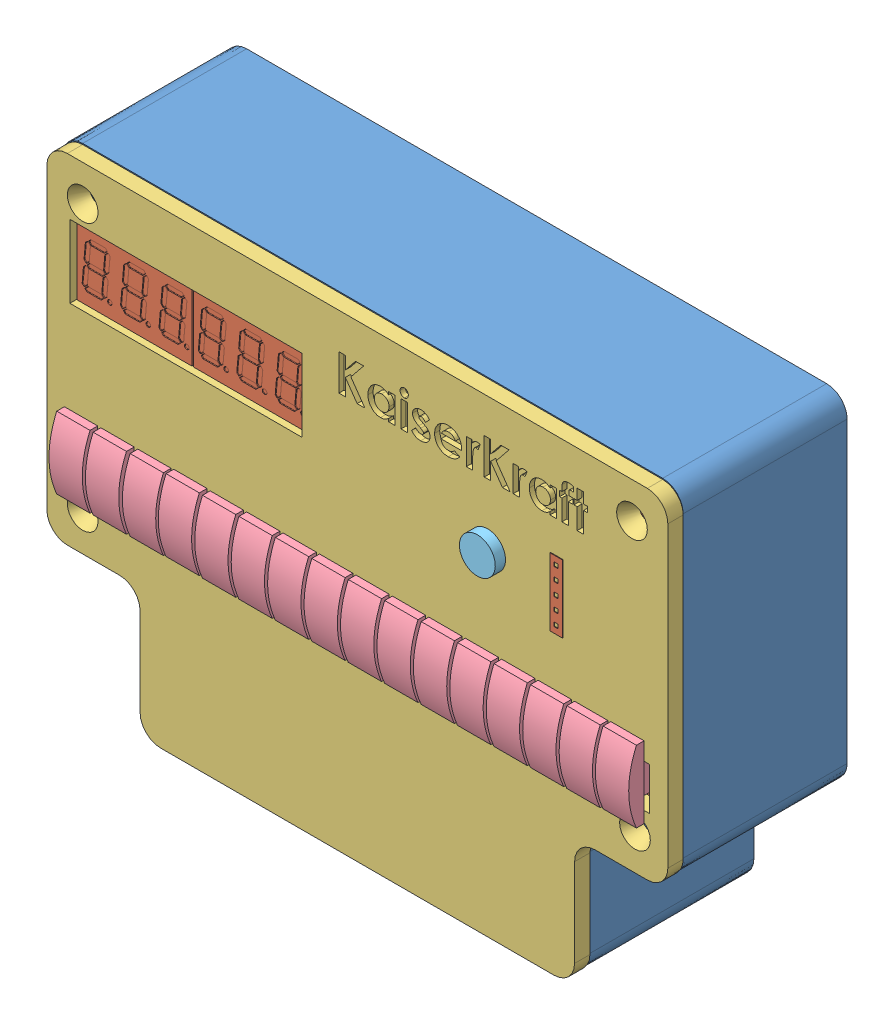
SolidWorks assembly submission, configuration Domyślna. Lengths in mm.
Overall size (121.28 91.6 38.61).
21 component instances, 6 part files, 60 mates.
Components (placement in the parent):
- Bottom_part-1: Bottom_part [Domyślna] x (-1 0 0) z (0 0 -1) size (121.2 91.4 32)
- Calculator.step-2: Calculator.step [Domyślna] at (-115.2 -0.196 -5.3886) size (120.85 86.07 32.47)
- Top_part-1: Top_part [Domyślna] at origin size (121.2 91.4 3)
- Switch_part-1: Switch_part [Domyślna] at (-111.9619 14.572 -0.3886) x (1 0 0) z (0 0 1) size (6.5 14 7)
- Switch_part-2: Switch_part [Domyślna] at (-104.8499 14.572 -0.3886) x (1 0 0) z (0 0 1) size (6.5 14 7)
- Button_top-1: Button_top [Domyślna] at (-31.5 37.75 5.6799) x (0.247537 0.968879 0) z (0 0 -1) size (7 7 6)
- Button_bottom-1: Button_bottom [Domyślna] at (-31.5 37.75 -0.3201) x (0.962619 -0.270858 0) z (0 0 1) size (5 5 2)
- Switch_part-5: Switch_part [Domyślna] at (-97.6379 14.572 -0.3886) x (1 0 0) z (0 0 1) size (6.5 14 7)
- Switch_part-6: Switch_part [Domyślna] at (-90.6259 14.672 -0.3886) x (1 0 0) z (0 0 1) size (6.5 14 7)
- Switch_part-7: Switch_part [Domyślna] at (-83.5139 14.572 -0.3886) x (1 0 0) z (0 0 1) size (6.5 14 7)
- Switch_part-8: Switch_part [Domyślna] at (-76.4019 14.572 -0.3886) x (1 0 0) z (0 0 1) size (6.5 14 7)
- Switch_part-9: Switch_part [Domyślna] at (-69.2899 14.572 -0.3886) x (1 0 0) z (0 0 1) size (6.5 14 7)
- Switch_part-10: Switch_part [Domyślna] at (-62.1779 14.572 -0.3886) x (1 0 0) z (0 0 1) size (6.5 14 7)
- Switch_part-11: Switch_part [Domyślna] at (-55.0659 14.572 -0.3886) x (1 0 0) z (0 0 1) size (6.5 14 7)
- Switch_part-12: Switch_part [Domyślna] at (-47.9539 14.572 -0.3886) x (1 0 0) z (0 0 1) size (6.5 14 7)
- Switch_part-13: Switch_part [Domyślna] at (-40.8419 14.572 -0.3886) x (1 0 0) z (0 0 1) size (6.5 14 7)
- Switch_part-14: Switch_part [Domyślna] at (-33.7299 14.572 -0.3886) x (1 0 0) z (0 0 1) size (6.5 14 7)
- Switch_part-15: Switch_part [Domyślna] at (-26.6179 14.572 -0.3886) x (1 0 0) z (0 0 1) size (6.5 14 7)
- Switch_part-16: Switch_part [Domyślna] at (-19.5059 14.572 -0.3886) x (1 0 0) z (0 0 1) size (6.5 14 7)
- Switch_part-17: Switch_part [Domyślna] at (-12.3939 14.572 -0.3886) x (1 0 0) z (0 0 1) size (6.5 14 7)
- Switch_part-18: Switch_part [Domyślna] at (-5.3219 14.672 -0.3886) x (1 0 0) z (0 0 1) size (6.5 14 7)
Mates (geometry in assembly coordinates):
- Wspólnie1: coincident: plane of Calculator.step-1 through (-48.0898 -16.8983 120.85) normal (0 0 1); circle of Bottom_part-1
- Wspólnie2: coincident: plane of Calculator.step-1 through (-48.0898 43.0977 120.4385) normal (-1 0 0); plane of Bottom_part-1 through (-115.2 60.2 -29) normal (1 0 0)
- Wspólnie3: coincident anti-aligned: plane of Calculator.step-1 through (66.9062 43.0977 120.4385) normal (0 1 0); plane of Bottom_part-1 through (0 60.2 -29) normal (0 -1 0)
- Ustalone2: in place: plane of ? through (66.9102 -16.9023 122.45) normal (0 0 1); plane of ? through (0 0 122.45) normal (0 0 1); moOrthogonalPlaneRef_w of ? through (66.9102 -16.9023 122.45) normal (0 0 1); plane of ? through (0 0 122.45) normal (0 1 0); plane of ? through (66.9102 -16.9023 122.45) normal (0 0 1); plane of ? through (0 0 122.45) normal (1 0 0); plane of Bottom_part-1 through (0 0 0) normal (0 0 1); unknown of Top_part-1
- Wspólnie9: coincident aligned: plane of Bottom_part-1; plane of Top_part-1
- Wspólnie10: coincident aligned: moOrthogonalPlaneRef_w of Bottom_part-1 through (0 0 0) normal (0 1 0); plane of Część6^submission-1 through (0 0 0) normal (0 1 0)
- Wspólnie11: coincident anti-aligned: moOrthogonalPlaneRef_w of Bottom_part-1 through (0 0 0) normal (-1 0 0); plane of Część6^submission-1 through (0 0 0) normal (1 0 0)
- Wspólnie18: coincident anti-aligned: plane of Bottom_part-1 through (-3.9013 56.1037 -7) normal (0 0 1); plane of Calculator.step-2 through (-115.2 -0.196 -7) normal (0 0 -1)
- Wspólnie19: coincident anti-aligned: plane of Bottom_part-1 through (-97 -25.2 -29) normal (0 1 0); plane of Calculator.step-2 through (-97.2 -25.2 -7) normal (0 -1 0)
- Wspólnie20: coincident: plane of Bottom_part-1 through (-115.2 60.2 -29) normal (1 0 0); line of Calculator.step-2 through (-115.2 59.8 -5.3886) axis (0 -1 0)
- Wspólnie21: coincident anti-aligned: plane of Calculator.step-2 through (-109.8619 17.1354 -0.3886) normal (1 0 0); plane of Switch_part-1 through (-109.8619 14.572 3.6114) normal (-1 0 0)
- Wspólnie24: coincident anti-aligned: plane of Calculator.step-2 through (-111.8619 13.072 3.6114) normal (0 0 1); plane of Switch_part-1 through (-111.9619 14.572 3.6114) normal (0 0 -1)
- Wspólnie25: coincident anti-aligned: plane of Calculator.step-2 through (-111.8619 14.572 -1.3886) normal (0 1 0); plane of Switch_part-1 through (-111.9619 14.572 3.6114) normal (0 -1 0)
- Wspólnie26: coincident anti-aligned: plane of Calculator.step-2 through (-102.7499 17.1354 -0.3886) normal (1 0 0); plane of Switch_part-2 through (-102.7499 14.572 3.6114) normal (-1 0 0)
- Wspólnie27: coincident anti-aligned: plane of Calculator.step-2 through (-104.7499 13.072 3.6114) normal (0 0 1); plane of Switch_part-2 through (-104.8499 14.572 3.6114) normal (0 0 -1)
- Wspólnie28: coincident anti-aligned: plane of Calculator.step-2 through (-104.7499 14.572 -1.3886) normal (0 1 0); plane of Switch_part-2 through (-104.8499 14.572 3.6114) normal (0 -1 0)
- Koncentryczne3: concentric anti-aligned: cylinder of Top_part-1 through (-31.5 37.75 0) axis (0 0 1) radius 1.6; cylinder of Button_bottom-1 through (-31.5 37.75 1.6799) axis (0 0 -1) radius 1.5
- Koncentryczne4: concentric anti-aligned: cylinder of Top_part-1 through (-31.5 37.75 0) axis (0 0 1) radius 1.6; circle of Button_top-1
- Wspólnie29: coincident aligned: circle of Button_top-1; plane of Button_bottom-1 through (-31.5 37.75 -0.3201) normal (0 0 -1)
- Wspólnie30: coincident anti-aligned: plane of Calculator.step-2 through (-97.6379 14.572 -1.3886) normal (0 1 0); plane of Switch_part-3 through (-82.5484 14.572 10.5) normal (0 -1 0)
- Wspólnie33: coincident anti-aligned: plane of Calculator.step-2 through (-96.2263 17.1354 -0.3886) normal (0 0 1); plane of Switch_part-5 through (-97.6379 14.572 -0.3886) normal (0 0 -1)
- Wspólnie34: coincident anti-aligned: plane of Calculator.step-2 through (-89.1143 17.1354 -0.3886) normal (0 0 1); plane of Switch_part-6 through (-90.6259 14.672 -0.3886) normal (0 0 -1)
- Wspólnie35: coincident anti-aligned: plane of Calculator.step-2 through (-82.0023 17.1354 -0.3886) normal (0 0 1); plane of Switch_part-7 through (-83.5139 14.572 -0.3886) normal (0 0 -1)
- Wspólnie38: coincident anti-aligned: plane of Calculator.step-2 through (-90.5259 12.572 3.6114) normal (0 -1 0); plane of Switch_part-6 through (-90.6259 12.572 3.6114) normal (0 1 0)
- Wspólnie39: coincident anti-aligned: plane of Calculator.step-2 through (-88.5259 17.1354 -0.3886) normal (1 0 0); plane of Switch_part-6 through (-88.5259 14.672 3.6114) normal (-1 0 0)
- Wspólnie41: coincident anti-aligned: plane of Calculator.step-2 through (-81.4139 17.1354 -0.3886) normal (1 0 0); plane of Switch_part-7 through (-81.4139 14.572 3.6114) normal (-1 0 0)
- Wspólnie42: coincident anti-aligned: plane of Calculator.step-2 through (-83.4139 14.572 -1.3886) normal (0 1 0); plane of Switch_part-7 through (-83.5139 14.572 3.6114) normal (0 -1 0)
- Wspólnie77: coincident anti-aligned: plane of Calculator.step-2 through (-3.8103 17.1354 -0.3886) normal (0 0 1); plane of Switch_part-18 through (-5.3219 14.672 -0.3886) normal (0 0 -1)
- Wspólnie78: coincident anti-aligned: plane of Calculator.step-2 through (-3.8103 17.1354 -0.3886) normal (0 0 1); plane of Switch_part-17 through (-12.3939 14.572 -0.3886) normal (0 0 -1)
- Wspólnie80: coincident anti-aligned: plane of Calculator.step-2 through (-3.8103 17.1354 -0.3886) normal (0 0 1); plane of Switch_part-16 through (-19.5059 14.572 -0.3886) normal (0 0 -1)
- Wspólnie81: coincident anti-aligned: plane of Calculator.step-2 through (-3.8103 17.1354 -0.3886) normal (0 0 1); plane of Switch_part-15 through (-26.6179 14.572 -0.3886) normal (0 0 -1)
- Wspólnie82: coincident anti-aligned: plane of Calculator.step-2 through (-3.8103 17.1354 -0.3886) normal (0 0 1); plane of Switch_part-14 through (-33.7299 14.572 -0.3886) normal (0 0 -1)
- Wspólnie83: coincident anti-aligned: plane of Calculator.step-2 through (-3.8103 17.1354 -0.3886) normal (0 0 1); plane of Switch_part-13 through (-40.8419 14.572 -0.3886) normal (0 0 -1)
- Wspólnie84: coincident anti-aligned: plane of Calculator.step-2 through (-3.8103 17.1354 -0.3886) normal (0 0 1); plane of Switch_part-12 through (-47.9539 14.572 -0.3886) normal (0 0 -1)
- Wspólnie85: coincident anti-aligned: plane of Calculator.step-2 through (-3.8103 17.1354 -0.3886) normal (0 0 1); plane of Switch_part-11 through (-55.0659 14.572 -0.3886) normal (0 0 -1)
- Wspólnie86: coincident anti-aligned: plane of Calculator.step-2 through (-3.8103 17.1354 -0.3886) normal (0 0 1); plane of Switch_part-10 through (-62.1779 14.572 -0.3886) normal (0 0 -1)
- Wspólnie87: coincident anti-aligned: plane of Calculator.step-2 through (-3.8103 17.1354 -0.3886) normal (0 0 1); plane of Switch_part-8 through (-76.4019 14.572 -0.3886) normal (0 0 -1)
- Wspólnie88: coincident anti-aligned: plane of Calculator.step-2 through (-3.8103 17.1354 -0.3886) normal (0 0 1); plane of Switch_part-9 through (-69.2899 14.572 -0.3886) normal (0 0 -1)
- Wspólnie89: coincident anti-aligned: plane of Calculator.step-2 through (-3.2219 17.1354 -0.3886) normal (1 0 0); plane of Switch_part-18 through (-3.2219 14.672 3.6114) normal (-1 0 0)
- Wspólnie90: coincident anti-aligned: plane of Calculator.step-2 through (-10.2939 17.1354 -0.3886) normal (1 0 0); plane of Switch_part-17 through (-10.2939 14.572 3.6114) normal (-1 0 0)
- Wspólnie91: coincident anti-aligned: plane of Calculator.step-2 through (-17.4059 17.1354 -0.3886) normal (1 0 0); plane of Switch_part-16 through (-17.4059 14.572 3.6114) normal (-1 0 0)
- Wspólnie92: coincident anti-aligned: plane of Calculator.step-2 through (-24.5179 17.1354 -0.3886) normal (1 0 0); plane of Switch_part-15 through (-24.5179 14.572 3.6114) normal (-1 0 0)
- Wspólnie93: coincident anti-aligned: plane of Calculator.step-2 through (-31.6299 17.1354 -0.3886) normal (1 0 0); plane of Switch_part-14 through (-31.6299 14.572 3.6114) normal (-1 0 0)
- Wspólnie94: coincident anti-aligned: plane of Calculator.step-2 through (-38.7419 17.1354 -0.3886) normal (1 0 0); plane of Switch_part-13 through (-38.7419 14.572 3.6114) normal (-1 0 0)
- Wspólnie95: coincident anti-aligned: plane of Calculator.step-2 through (-45.8539 17.1354 -0.3886) normal (1 0 0); plane of Switch_part-12 through (-45.8539 14.572 3.6114) normal (-1 0 0)
- Wspólnie96: coincident anti-aligned: plane of Calculator.step-2 through (-52.9659 17.1354 -0.3886) normal (1 0 0); plane of Switch_part-11 through (-52.9659 14.572 3.6114) normal (-1 0 0)
- Wspólnie97: coincident anti-aligned: plane of Calculator.step-2 through (-60.0779 17.1354 -0.3886) normal (1 0 0); plane of Switch_part-10 through (-60.0779 14.572 3.6114) normal (-1 0 0)
- Wspólnie98: coincident anti-aligned: plane of Calculator.step-2 through (-67.1899 17.1354 -0.3886) normal (1 0 0); plane of Switch_part-9 through (-67.1899 14.572 3.6114) normal (-1 0 0)
- Wspólnie99: coincident anti-aligned: plane of Calculator.step-2 through (-74.3019 17.1354 -0.3886) normal (1 0 0); plane of Switch_part-8 through (-74.3019 14.572 3.6114) normal (-1 0 0)
- Wspólnie100: coincident anti-aligned: plane of Calculator.step-2 through (-5.2219 12.572 3.6114) normal (0 -1 0); plane of Switch_part-18 through (-5.3219 12.572 3.6114) normal (0 1 0)
- Wspólnie101: coincident anti-aligned: plane of Calculator.step-2 through (-12.2939 14.572 -1.3886) normal (0 1 0); plane of Switch_part-17 through (-12.3939 14.572 3.6114) normal (0 -1 0)
- Wspólnie102: coincident anti-aligned: plane of Calculator.step-2 through (-19.4059 14.572 -1.3886) normal (0 1 0); plane of Switch_part-16 through (-19.5059 14.572 3.6114) normal (0 -1 0)
- Wspólnie103: coincident anti-aligned: plane of Calculator.step-2 through (-26.5179 14.572 -1.3886) normal (0 1 0); plane of Switch_part-15 through (-26.6179 14.572 3.6114) normal (0 -1 0)
- Wspólnie104: coincident anti-aligned: plane of Calculator.step-2 through (-33.6299 14.572 -1.3886) normal (0 1 0); plane of Switch_part-14 through (-33.7299 14.572 3.6114) normal (0 -1 0)
- Wspólnie105: coincident anti-aligned: plane of Calculator.step-2 through (-40.7419 14.572 -1.3886) normal (0 1 0); plane of Switch_part-13 through (-40.8419 14.572 3.6114) normal (0 -1 0)
- Wspólnie106: coincident anti-aligned: plane of Calculator.step-2 through (-47.8539 14.572 -1.3886) normal (0 1 0); plane of Switch_part-12 through (-47.9539 14.572 3.6114) normal (0 -1 0)
- Wspólnie107: coincident anti-aligned: plane of Calculator.step-2 through (-54.9659 14.572 -1.3886) normal (0 1 0); plane of Switch_part-11 through (-55.0659 14.572 3.6114) normal (0 -1 0)
- Wspólnie108: coincident anti-aligned: plane of Calculator.step-2 through (-62.0779 14.572 -1.3886) normal (0 1 0); plane of Switch_part-10 through (-62.1779 14.572 3.6114) normal (0 -1 0)
- Wspólnie109: coincident anti-aligned: plane of Calculator.step-2 through (-69.1899 14.572 -1.3886) normal (0 1 0); plane of Switch_part-9 through (-69.2899 14.572 3.6114) normal (0 -1 0)
- Wspólnie110: coincident anti-aligned: plane of Calculator.step-2 through (-76.3019 14.572 -1.3886) normal (0 1 0); plane of Switch_part-8 through (-76.4019 14.572 3.6114) normal (0 -1 0)
